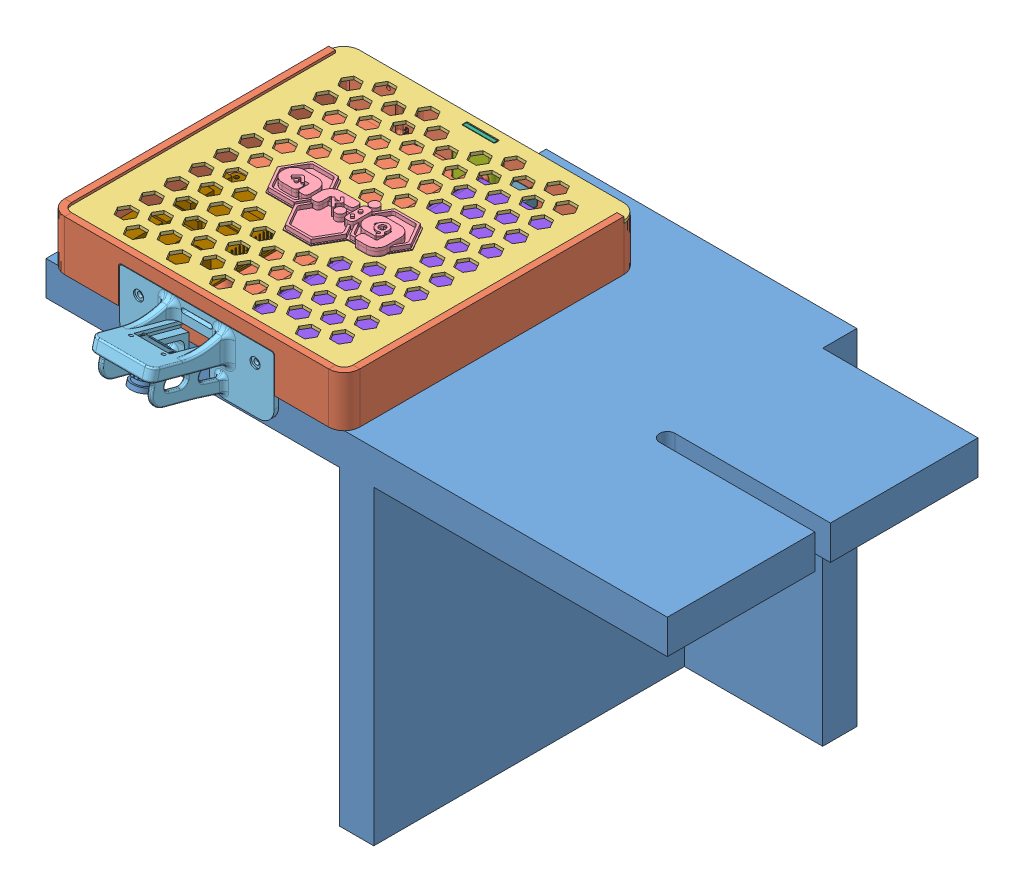
SolidWorks assembly assembly, configuration Défaut. Lengths in mm.
Overall size (400 254.4 276.81).
60 component instances, 38 part files, 9 mates.
Components (placement in the parent):
- support-1: support [Défaut] at (0 -22 0) size (400 222 222)
- vision-1: vision [Défaut] at (-100 0 108) x (0 0 1) z (-1 0 0) size (246.21 50.4 190)
  - box-1: box [Défaut] at origin size (190.6 32.4 190)
  - cover-1: cover [Défaut] at (-1.3 28.3 0) x (0 0 1) z (-1 0 0) size (190 2 187) (hidden)
  - LogoARIG2-1: LogoARIG2 [Défaut] at (29.3179 30.3 42.8) x (0 0 -1) z (0 1 0) size (88.08 45.8 6.03) (hidden)
  - support-cam-1: support-cam [Défaut] at (92 2.85 0) x (0 0 -1) z (1 0 0) size (99.5 41.7 53.04)
  - latch-1: latch [Défaut] at (-84.4 7.063 -10) size (14.06 23.3 20)
  - latch-box-1: latch-box [Défaut] at (-81.6 1.6 0) x (0 0 -1) z (1 0 0) size (26.6 26.5 9)
  - Xiaomi PowerBank-1: Xiaomi PowerBank [Défaut] at (84.75 2.8 -89.15) x (0 0 1) z (-1 0 0) size (70 25 150)
  - raspberryPi3BSimplified_STEP.step-1: raspberryPi3BSimplified_STEP.step [Défaut] at (32.5 6.8 51.4) x (1 0 0) z (0 1 0) size (87 58.5 18.55)
  - OSSD-128x64.igs-1: OSSD-128x64.igs [Défaut] at (-91.9 15.3 69.5) x (0 0 1) z (0 -1 0) size (25 5.1 26)
  - micro push button-2: micro push button [Défaut] at (-89.5 6.8667 45.1) x (0 -1 0) z (0 0 -1) size (5.8 13.4 5.8)
  - mini swich-1: mini swich [Défaut] at (-89.9 19.2833 45.2) x (0 1 0) z (0 0 1) size (10.5 12.4 5.6)
  - spring-1: spring [Défaut] at (-87.002 2.3106 6.0058) x (0.974863 -0.040201 -0.21915) z (0.219381 0.001367 0.975638) size (4.02 10.6 4.01)
  - spring-2: spring [Défaut] at (-87.0662 11.9402 -5.894) x (-0.826432 0.000175 -0.563036) z (-0.56297 -0.015546 0.826331) size (4.02 10.6 4.01)
  - usb-port-1: usb-port [Défaut] at (-65.85 15.3 -33.65) x (0 0 1) z (-1 0 0) size (15.2 7.3 34.7)
  - RspCameraMia-1: RspCameraMia [Défaut] at (130.1784 16.2188 -0.0942) x (0.965926 0.258819 0) z (0.258819 -0.965926 0) size (23.86 25 22.7)
    - RspCameraMia.stp-1: RspCameraMia.stp [Défaut] at origin size (23.86 25 9.96)
      - 70521906.stp-1: 70521906.stp [Défaut] at (1.7167 0.8597 0.0159) size (2 2.1 0.95)
        - 70521906_01.stp-1: 70521906_01.stp [Défaut] at origin size (0.25 0.55 0.75)
        - 70521906_02.stp-1: 70521906_02.stp [Défaut] at origin size (0.25 0.55 0.75)
        - 70521906_03.stp-1: 70521906_03.stp [Défaut] at origin size (2 1.25 0.9)
        - 70521906_04.stp-1: 70521906_04.stp [Défaut] at origin size (0.25 0.55 0.75)
        - 70521906_05.stp-1: 70521906_05.stp [Défaut] at origin size (0.25 0.55 0.75)
        - 70521906_06.stp-1: 70521906_06.stp [Défaut] at origin size (0.25 0.55 0.75)
        - 70521906_07.stp-1: 70521906_07.stp [Défaut] at origin size (0.25 0.55 0.75)
      - PicameraPCB.stp-1: PicameraPCB.stp [Défaut] at (0.2393 -0.0199 0) x (-1 0 0) z (0 0 1) size (23.86 25 2.2)
      - OVA5647_Housing.stp-1: OVA5647_Housing.stp [Défaut] at (-2.4078 0.0859 1) x (1 0 0) z (0 -1 0) size (8 3.95 8)
      - OVA5647_Lens_FOV.stp-1: OVA5647_Lens_FOV.stp [Défaut] at (-2.4087 0.0921 5.963) x (1 0 0) z (0 -1 0) size (6 3.35 6)
      - ribbon_cam.stp-1: ribbon_cam.stp [Défaut] at (-2.4804 0.3633 1.4162) x (0 1 0) z (1 0 0) size (5.6 0.69 4.76)
      - CCD.stp-1: CCD.stp [Défaut] at (-2.0757 0.287 1.296) x (1 0 0) z (0 -1 0) size (8.01 0.69 8.01)
      - CAPC-0805-T0.75-BN.stp-1: CAPC-0805-T0.75-BN.stp [Défaut] at (4.562 5.9833 -0.0026) x (0 -1 0) z (0 0 -1) size (2.1 1.35 0.75)
      - CAPC-0805-T0.75-BN.stp-2: CAPC-0805-T0.75-BN.stp [Défaut] at (2.0233 10.2705 -0.0026) x (0 -1 0) z (0 0 -1) size (2.1 1.35 0.75)
      - CAPC-0402-T0.55-BN.stp-1: CAPC-0402-T0.55-BN.stp [Défaut] at (-2.9562 6.224 -0.2572) x (-1 0 0) z (0 -1 0) size (1.05 0.55 0.55)
      - CAPC-0402-T0.55-BN.stp-2: CAPC-0402-T0.55-BN.stp [Défaut] at (-2.9504 5.2898 -0.2691) x (-1 0 0) z (0 -1 0) size (1.05 0.55 0.55)
      - CAPC-0402-T0.55-BN.stp-3: CAPC-0402-T0.55-BN.stp [Défaut] at (4.5768 -5.1833 -0.2811) x (-1 0 0) z (0 -1 0) size (1.05 0.55 0.55)
      - CAPC-0402-T0.55-BN.stp-4: CAPC-0402-T0.55-BN.stp [Défaut] at (2.5547 -5.1368 -0.2811) x (-1 0 0) z (0 -1 0) size (1.05 0.55 0.55)
      - CAPC-0402-T0.55-BN.stp-5: CAPC-0402-T0.55-BN.stp [Défaut] at (2.6129 -9.93 -0.293) x (-1 0 0) z (0 -1 0) size (1.05 0.55 0.55)
      - CAPC-0402-T0.55-BN.stp-6: CAPC-0402-T0.55-BN.stp [Défaut] at (4.7286 -9.9294 -0.293) x (-1 0 0) z (0 -1 0) size (1.05 0.55 0.55)
      - CAPC-0402-T0.55-BN.stp-7: CAPC-0402-T0.55-BN.stp [Défaut] at (8.4068 -3.8793 -0.2811) x (-1 0 0) z (0 -1 0) size (1.05 0.55 0.55)
      - CAPC-0402-T0.55-BN.stp-8: CAPC-0402-T0.55-BN.stp [Défaut] at (9.0088 0.0217 -0.2796) x (0 1 0) z (-1 0 0) size (1.05 0.55 0.55)
      - CAPC-0402-T0.55-BN.stp-9: CAPC-0402-T0.55-BN.stp [Défaut] at (10.4284 2.6731 -0.3022) x (0 1 0) z (-1 0 0) size (1.05 0.55 0.55)
      - CAPC-0402-T0.55-BN.stp-10: CAPC-0402-T0.55-BN.stp [Défaut] at (8.2321 1.3259 -0.2838) x (1 0 0) z (0 1 0) size (1.05 0.55 0.55)
      - RESC-0402.stp-1: RESC-0402.stp [Défaut] at (3.7919 0.0148 -0.0114) x (1 0 0) z (0 0 -1) size (1.05 0.55 0.4)
      - RESC-0402.stp-2: RESC-0402.stp [Défaut] at (4.1232 2.6296 -0.0028) x (0 -1 0) z (0 0 -1) size (1.05 0.55 0.4)
      - RESC-0402.stp-3: RESC-0402.stp [Défaut] at (10.5883 -6.2795 -0.0019) x (0 1 0) z (0 0 -1) size (1.05 0.55 0.4)
      - RESC-0603.stp-1: RESC-0603.stp [Défaut] at (-2.6191 7.0617 -0.0121) x (1 0 0) z (0 0 -1) size (1.7 0.9 0.55)
      - RESC-0603.stp-2: RESC-0603.stp [Défaut] at (-3.4466 3.0018 -0.0048) x (0 -1 0) z (0 0 -1) size (1.7 0.9 0.55)
      - RESC-1210.stp-1: RESC-1210.stp [Défaut] at (2.2265 5.9002 -0.0068) x (0 -1 0) z (0 0 -1) size (3.3 2.7 0.6)
      - c-1-1734248-5-e-raspberry_display.stp-1: c-1-1734248-5-e-raspberry_display.stp [Défaut] at (-10.6651 0.0449 -1.5) x (0 -1 0) z (-1 0 0) size (22.4 3.22 5.68)
      - SOT23-5.stp-1: SOT23-5.stp [Défaut] at (4.2989 9.8879 0.5457) x (0 -1 0) z (0 0 -1) size (2.84 3.03 1.19)
      - SOT23-5.stp-2: SOT23-5.stp [Défaut] at (3.5194 -3.2493 0.04) x (-1 0 0) z (0 0 -1) size (2.84 3.03 1.19)
      - SOT23-5.stp-3: SOT23-5.stp [Défaut] at (3.5816 -8.055 0.0206) x (-1 0 0) z (0 0 -1) size (2.84 3.03 1.19)
      - KX7 SMD Quartz Crystal Resonator 3.2x2.5mm.stp-1: KX7 SMD Quartz Crystal Resonator 3.2x2.5mm.stp [Défaut] at (9.9746 -4.9221 0.0339) x (-1 0 0) z (0 -1 0) size (3.2 0.6 2.5)
      - c6aaa.stp-1: c6aaa.stp [Défaut] at (0.0643 0.0942 0) x (1 0 0) z (0 0 -1) size (2 2.99 0.6)
      - 4pin_smd.stp-1: 4pin_smd.stp [Défaut] at (0.027 0.0676 0) x (1 0 0) z (0 0 -1) size (1.29 1 0.47)
      - 4pin_smd.stp-2: 4pin_smd.stp [Défaut] at (-0.0093 -6.0092 -0.0198) x (1 0 0) z (0 0 -1) size (1.29 1 0.47)
      - 4pin_smd.stp-3: 4pin_smd.stp [Défaut] at (0.0326 -3.0068 -0.0235) x (1 0 0) z (0 0 -1) size (1.29 1 0.47)
    - WideAngleLens.step-1: WideAngleLens.step [Défaut] at (-4.3167 0.0942 2.6) x (1 0 0) z (0 -1 0) size (14 16.9 14)
  - central-nut-1: central-nut [Défaut] at (-8 2.8 0) x (0 0 -1) z (1 0 0) size (34 10.5 36) (hidden)
Mates (geometry in assembly coordinates):
- Coïncidente4: coincident: plane of support-1 through (-200 0 0) normal (0 0 -1); plane of assembly through (0 0 0) normal (0 0 1)
- Coïncidente5: coincident: plane of support-1 through (-100 0 100) normal (0 1 0); plane of assembly through (0 0 0) normal (0 1 0)
- Coïncidente6: coincident: moEndPointRef_w of support-1; plane of assembly
- Coaxiale1: concentric: circle of support-1; circle of ?
- Coïncidente8: coincident: plane of support-1 through (-100 0 100) normal (0 1 0); plane of ? through (-89.262 0 96.3263) normal (0 -1 0)
- Parallèle2: parallel: plane of support-1 through (0 0 200) normal (0 0 1); plane of ? through (-11 27.3 200) normal (0 0 1)
- Coïncidente9: coincident: plane of support-1 through (-100 0 100) normal (0 1 0); plane of vision-1/box-1 through (-100 0 108) normal (0 -1 0)
- Parallèle3: parallel: plane of support-1 through (0 0 200) normal (0 0 1); plane of vision-1/box-1 through (-5 28.3 203) normal (0 0 1)
- Coaxiale2: concentric: cylinder of support-1 through (-100 0 100) axis (0 -1 0) radius 5; cylinder of vision-1/box-1 through (-100 28.3 100) axis (0 -1 0) radius 4
